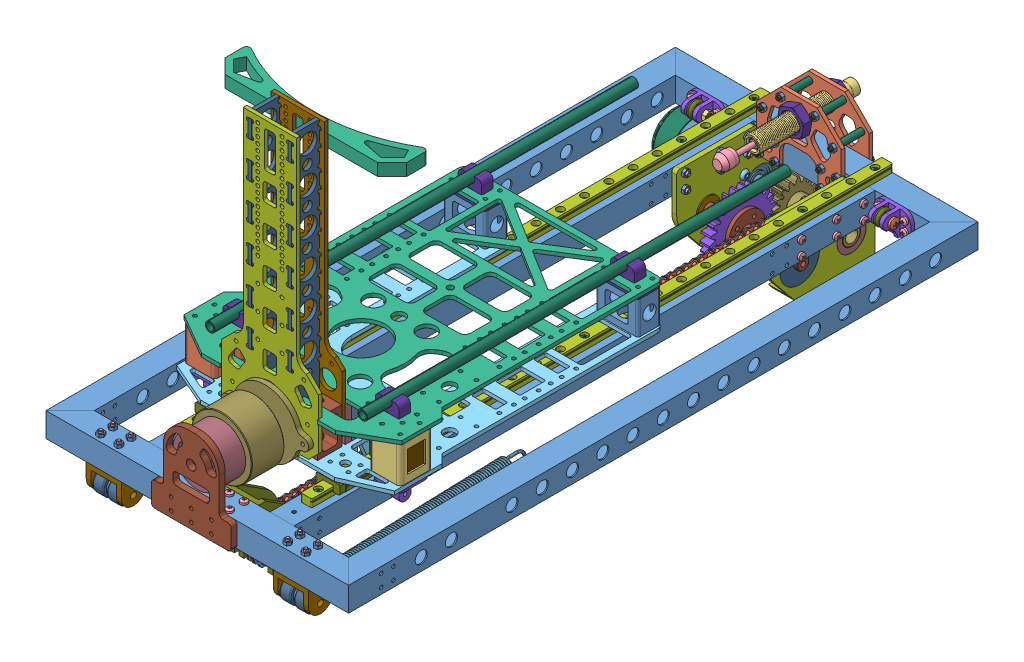
SolidWorks assembly 寒冰射手-wlⅡ-2AT-sc, configuration 默认. Lengths in mm. (continued)
Mates (geometry in assembly coordinates): (continued)
- 同心85: concentric anti-aligned: cylinder of 发射架-wlⅡ-2AT-sc-1 through (-111.2492 36.8186 -178.5) axis (1 0 0) radius 1.5; cylinder of GB／T818-2000十字槽盘头螺钉M3×28-wlⅡ-2AT-sc-7 through (-114.981 36.8186 -178.5) axis (-1 0 0) radius 1.5
- 重合126: coincident anti-aligned: plane of 发射架-wlⅡ-2AT-sc-1 through (-111.2492 32.8186 250) normal (-1 0 0); plane of GB／T818-2000十字槽盘头螺钉M3×28-wlⅡ-2AT-sc-7 through (-111.2492 38.6176 -178.4412) normal (1 0 0)
- 同心86: concentric anti-aligned: cylinder of 发射架-wlⅡ-2AT-sc-1 through (-111.2492 48.8186 -178.5) axis (1 0 0) radius 1.5; cylinder of GB／T818-2000十字槽盘头螺钉M3×28-wlⅡ-2AT-sc-8 through (-114.981 48.8186 -178.5) axis (-1 0 0) radius 1.5
- 同心87: concentric anti-aligned: cylinder of 发射架-wlⅡ-2AT-sc-1 through (-111.2492 48.8186 -207.5) axis (1 0 0) radius 1.5; cylinder of GB／T818-2000十字槽盘头螺钉M3×28-wlⅡ-2AT-sc-10 through (-114.981 48.8186 -207.5) axis (-1 0 0) radius 1.5
- 重合129: coincident anti-aligned: plane of 发射架-wlⅡ-2AT-sc-1 through (-111.2492 32.8186 250) normal (-1 0 0); plane of GB／T818-2000十字槽盘头螺钉M3×28-wlⅡ-2AT-sc-10 through (-111.2492 50.6176 -207.4412) normal (1 0 0)
- 重合130: coincident anti-aligned: plane of 发射架-wlⅡ-2AT-sc-1 through (-111.2492 32.8186 250) normal (-1 0 0); plane of GB／T818-2000十字槽盘头螺钉M3×28-wlⅡ-2AT-sc-8 through (-111.2492 50.6176 -178.4412) normal (1 0 0)
- 同心88: concentric anti-aligned: cylinder of 发射架-wlⅡ-2AT-sc-1 through (-111.2492 36.8186 -207.5) axis (1 0 0) radius 1.5; cylinder of GB／T818-2000十字槽盘头螺钉M3×28-wlⅡ-2AT-sc-9 through (-114.981 36.8186 -207.5) axis (-1 0 0) radius 1.5
- 重合131: coincident anti-aligned: plane of 发射架-wlⅡ-2AT-sc-1 through (-111.2492 32.8186 250) normal (-1 0 0); plane of GB／T818-2000十字槽盘头螺钉M3×28-wlⅡ-2AT-sc-9 through (-111.2492 38.6176 -207.4412) normal (1 0 0)
- 同心89: concentric anti-aligned: cylinder of 发射架-wlⅡ-2AT-sc-1 through (-111.2492 48.8186 -230) axis (1 0 0) radius 1.5; cylinder of GB／T818-2000十字槽盘头螺钉M3×28-wlⅡ-2AT-sc-11 through (-114.981 48.8186 -230) axis (-1 0 0) radius 1.5
- 重合132: coincident anti-aligned: plane of 发射架-wlⅡ-2AT-sc-1 through (-111.2492 32.8186 250) normal (-1 0 0); plane of GB／T818-2000十字槽盘头螺钉M3×28-wlⅡ-2AT-sc-11 through (-111.2492 50.6176 -230.0576) normal (1 0 0)
- 同心90: concentric anti-aligned: cylinder of 发射架-wlⅡ-2AT-sc-1 through (-111.2492 36.8186 -230) axis (1 0 0) radius 1.5; cylinder of GB／T818-2000十字槽盘头螺钉M3×28-wlⅡ-2AT-sc-12 through (-114.981 36.8186 -230) axis (-1 0 0) radius 1.5
- 重合133: coincident anti-aligned: plane of 发射架-wlⅡ-2AT-sc-1 through (-111.2492 32.8186 250) normal (-1 0 0); plane of GB／T818-2000十字槽盘头螺钉M3×28-wlⅡ-2AT-sc-12 through (-111.2492 38.6176 -229.9412) normal (1 0 0)
- 同心91: concentric anti-aligned: cylinder of GB／T818-2000十字槽盘头螺钉M3×28-wlⅡ-2AT-sc-1 through (12.4826 48.8186 -230) axis (1 0 0) radius 1.5; cylinder of GB／T6170-20001型六角螺母A级和B级M3-wlⅡ-2AT-sc-15 through (-15.2492 48.8186 -230) axis (-1 0 0) radius 1.5
- 同心92: concentric anti-aligned: cylinder of GB／T818-2000十字槽盘头螺钉M3×28-wlⅡ-2AT-sc-2 through (12.4826 36.8186 -230) axis (1 0 0) radius 1.5; cylinder of GB／T6170-20001型六角螺母A级和B级M3-wlⅡ-2AT-sc-16 through (-15.2492 36.8186 -230) axis (-1 0 0) radius 1.5
- 同心93: concentric anti-aligned: cylinder of GB／T818-2000十字槽盘头螺钉M3×28-wlⅡ-2AT-sc-3 through (12.4826 36.8186 -207.5) axis (1 0 0) radius 1.5; cylinder of GB／T6170-20001型六角螺母A级和B级M3-wlⅡ-2AT-sc-18 through (-15.2492 36.8186 -207.5) axis (-1 0 0) radius 1.5
- 同心94: concentric anti-aligned: cylinder of GB／T818-2000十字槽盘头螺钉M3×28-wlⅡ-2AT-sc-4 through (12.4826 48.8186 -207.5) axis (1 0 0) radius 1.5; cylinder of GB／T6170-20001型六角螺母A级和B级M3-wlⅡ-2AT-sc-17 through (-15.2492 48.8186 -207.5) axis (-1 0 0) radius 1.5
- 同心95: concentric anti-aligned: cylinder of GB／T818-2000十字槽盘头螺钉M3×28-wlⅡ-2AT-sc-6 through (12.4826 36.8186 -178.5) axis (1 0 0) radius 1.5; cylinder of GB／T6170-20001型六角螺母A级和B级M3-wlⅡ-2AT-sc-20 through (-15.2492 36.8186 -178.5) axis (-1 0 0) radius 1.5
- 同心96: concentric anti-aligned: cylinder of GB／T818-2000十字槽盘头螺钉M3×28-wlⅡ-2AT-sc-5 through (12.4826 48.8186 -178.5) axis (1 0 0) radius 1.5; cylinder of GB／T6170-20001型六角螺母A级和B级M3-wlⅡ-2AT-sc-19 through (-15.2492 48.8186 -178.5) axis (-1 0 0) radius 1.5
- 同心97: concentric aligned: cylinder of GB／T818-2000十字槽盘头螺钉M3×28-wlⅡ-2AT-sc-8 through (-114.981 48.8186 -178.5) axis (-1 0 0) radius 1.5; cylinder of GB／T6170-20001型六角螺母A级和B级M3-wlⅡ-2AT-sc-21 through (-84.8492 48.8186 -178.5) axis (-1 0 0) radius 1.5
- 同心98: concentric aligned: cylinder of GB／T818-2000十字槽盘头螺钉M3×28-wlⅡ-2AT-sc-7 through (-114.981 36.8186 -178.5) axis (-1 0 0) radius 1.5; cylinder of GB／T6170-20001型六角螺母A级和B级M3-wlⅡ-2AT-sc-23 through (-84.8492 36.8186 -178.5) axis (-1 0 0) radius 1.5
- 同心99: concentric aligned: cylinder of GB／T818-2000十字槽盘头螺钉M3×28-wlⅡ-2AT-sc-9 through (-114.981 36.8186 -207.5) axis (-1 0 0) radius 1.5; cylinder of GB／T6170-20001型六角螺母A级和B级M3-wlⅡ-2AT-sc-28 through (-84.8492 36.8186 -207.5) axis (-1 0 0) radius 1.5
- 同心100: concentric aligned: cylinder of GB／T818-2000十字槽盘头螺钉M3×28-wlⅡ-2AT-sc-10 through (-114.981 48.8186 -207.5) axis (-1 0 0) radius 1.5; cylinder of GB／T6170-20001型六角螺母A级和B级M3-wlⅡ-2AT-sc-26 through (-84.8492 48.8186 -207.5) axis (-1 0 0) radius 1.5
- 同心101: concentric aligned: cylinder of GB／T818-2000十字槽盘头螺钉M3×28-wlⅡ-2AT-sc-11 through (-114.981 48.8186 -230) axis (-1 0 0) radius 1.5; cylinder of GB／T6170-20001型六角螺母A级和B级M3-wlⅡ-2AT-sc-27 through (-84.8492 48.8186 -230) axis (-1 0 0) radius 1.5
- 同心102: concentric aligned: cylinder of GB／T818-2000十字槽盘头螺钉M3×28-wlⅡ-2AT-sc-12 through (-114.981 36.8186 -230) axis (-1 0 0) radius 1.5; cylinder of GB／T6170-20001型六角螺母A级和B级M3-wlⅡ-2AT-sc-24 through (-84.8492 36.8186 -230) axis (-1 0 0) radius 1.5
- 同心107: concentric anti-aligned: cylinder of 拉线座子-wlⅡ-2AT-sc-2 through (-117.7492 46.8186 -237) axis (0 0 -1) radius 1.5; cylinder of GB／T818-2000十字槽盘头螺钉M3×28-wlⅡ-2AT-sc-13 through (-117.7492 46.8186 -233.2682) axis (0 0 1) radius 1.5
- 重合153: coincident anti-aligned: plane of 拉线座子-wlⅡ-2AT-sc-2 through (-128.4992 25.8186 -237) normal (0 0 1); plane of GB／T818-2000十字槽盘头螺钉M3×28-wlⅡ-2AT-sc-13 through (-118.3588 48.5122 -237) normal (0 0 -1)
- 同心108: concentric anti-aligned: cylinder of 拉线座子-wlⅡ-2AT-sc-2 through (-139.2492 46.8186 -237) axis (0 0 -1) radius 1.5; cylinder of GB／T818-2000十字槽盘头螺钉M3×28-wlⅡ-2AT-sc-16 through (-139.2492 46.8186 -233.2682) axis (0 0 1) radius 1.5
- 同心109: concentric anti-aligned: cylinder of 拉线座子-wlⅡ-2AT-sc-2 through (-139.2492 38.8186 -237) axis (0 0 -1) radius 1.5; cylinder of GB／T818-2000十字槽盘头螺钉M3×28-wlⅡ-2AT-sc-14 through (-139.2492 38.8186 -233.2682) axis (0 0 1) radius 1.5
- 同心110: concentric anti-aligned: cylinder of 拉线座子-wlⅡ-2AT-sc-2 through (-117.7492 38.8186 -237) axis (0 0 -1) radius 1.5; cylinder of GB／T818-2000十字槽盘头螺钉M3×28-wlⅡ-2AT-sc-15 through (-117.7492 38.8186 -233.2682) axis (0 0 1) radius 1.5
- 重合154: coincident anti-aligned: plane of 拉线座子-wlⅡ-2AT-sc-2 through (-128.4992 25.8186 -237) normal (0 0 1); plane of GB／T818-2000十字槽盘头螺钉M3×28-wlⅡ-2AT-sc-15 through (-118.3588 40.5122 -237) normal (0 0 -1)
- 重合155: coincident anti-aligned: plane of 拉线座子-wlⅡ-2AT-sc-2 through (-128.4992 25.8186 -237) normal (0 0 1); plane of GB／T818-2000十字槽盘头螺钉M3×28-wlⅡ-2AT-sc-16 through (-139.8588 48.5122 -237) normal (0 0 -1)
- 重合156: coincident anti-aligned: plane of 拉线座子-wlⅡ-2AT-sc-2 through (-128.4992 25.8186 -237) normal (0 0 1); plane of GB／T818-2000十字槽盘头螺钉M3×28-wlⅡ-2AT-sc-14 through (-139.8588 40.5122 -237) normal (0 0 -1)
- 同心111: concentric anti-aligned: cylinder of 拉线座子-wlⅡ-2AT-sc-1 through (15.2508 46.8186 -237) axis (0 0 -1) radius 1.5; cylinder of GB／T818-2000十字槽盘头螺钉M3×28-wlⅡ-2AT-sc-17 through (15.2508 46.8186 -233.2682) axis (0 0 1) radius 1.5
- 同心112: concentric anti-aligned: cylinder of 拉线座子-wlⅡ-2AT-sc-1 through (15.2508 38.8186 -237) axis (0 0 -1) radius 1.5; cylinder of GB／T818-2000十字槽盘头螺钉M3×28-wlⅡ-2AT-sc-19 through (15.2508 38.8186 -233.2682) axis (0 0 1) radius 1.5
- 同心113: concentric anti-aligned: cylinder of 拉线座子-wlⅡ-2AT-sc-1 through (36.7508 38.8186 -237) axis (0 0 -1) radius 1.5; cylinder of GB／T818-2000十字槽盘头螺钉M3×28-wlⅡ-2AT-sc-20 through (36.7508 38.8186 -233.2682) axis (0 0 1) radius 1.5
- 同心114: concentric anti-aligned: cylinder of 拉线座子-wlⅡ-2AT-sc-1 through (36.7508 46.8186 -237) axis (0 0 -1) radius 1.5; cylinder of GB／T818-2000十字槽盘头螺钉M3×28-wlⅡ-2AT-sc-18 through (36.7508 46.8186 -233.2682) axis (0 0 1) radius 1.5
- 重合157: coincident anti-aligned: plane of 拉线座子-wlⅡ-2AT-sc-1 through (26.0008 25.8186 -237) normal (0 0 1); plane of GB／T818-2000十字槽盘头螺钉M3×28-wlⅡ-2AT-sc-19 through (14.6412 40.5122 -237) normal (0 0 -1)
- 重合158: coincident anti-aligned: plane of 拉线座子-wlⅡ-2AT-sc-1 through (26.0008 25.8186 -237) normal (0 0 1); plane of GB／T818-2000十字槽盘头螺钉M3×28-wlⅡ-2AT-sc-18 through (36.1412 48.5122 -237) normal (0 0 -1)
- 重合159: coincident anti-aligned: plane of 拉线座子-wlⅡ-2AT-sc-1 through (26.0008 25.8186 -237) normal (0 0 1); plane of GB／T818-2000十字槽盘头螺钉M3×28-wlⅡ-2AT-sc-20 through (36.1412 40.5122 -237) normal (0 0 -1)
- 同心115: concentric anti-aligned: cylinder of GB／T818-2000十字槽盘头螺钉M3×28-wlⅡ-2AT-sc-20 through (36.7508 38.8186 -233.2682) axis (0 0 1) radius 1.5; cylinder of GB／T6170-20001型六角螺母A级和B级M3-wlⅡ-2AT-sc-29 through (36.7508 38.8186 -260) axis (0 0 -1) radius 1.5
- 重合160: coincident anti-aligned: plane of 发射架-wlⅡ-2AT-sc-1 through (63.7508 32.8186 -260) normal (0 0 -1); plane of GB／T6170-20001型六角螺母A级和B级M3-wlⅡ-2AT-sc-29 through (33.7458 38.8186 -260) normal (0 0 1)
- 同心116: concentric anti-aligned: cylinder of GB／T818-2000十字槽盘头螺钉M3×28-wlⅡ-2AT-sc-18 through (36.7508 46.8186 -233.2682) axis (0 0 1) radius 1.5; cylinder of GB／T6170-20001型六角螺母A级和B级M3-wlⅡ-2AT-sc-30 through (36.7508 46.8186 -260) axis (0 0 -1) radius 1.5
- 重合161: coincident anti-aligned: plane of 发射架-wlⅡ-2AT-sc-1 through (63.7508 32.8186 -260) normal (0 0 -1); plane of GB／T6170-20001型六角螺母A级和B级M3-wlⅡ-2AT-sc-30 through (33.7458 46.8186 -260) normal (0 0 1)
- 同心117: concentric anti-aligned: cylinder of GB／T818-2000十字槽盘头螺钉M3×28-wlⅡ-2AT-sc-19 through (15.2508 38.8186 -233.2682) axis (0 0 1) radius 1.5; cylinder of GB／T6170-20001型六角螺母A级和B级M3-wlⅡ-2AT-sc-31 through (15.2508 38.8186 -260) axis (0 0 -1) radius 1.5
- 同心118: concentric anti-aligned: cylinder of GB／T818-2000十字槽盘头螺钉M3×28-wlⅡ-2AT-sc-17 through (15.2508 46.8186 -233.2682) axis (0 0 1) radius 1.5; cylinder of GB／T6170-20001型六角螺母A级和B级M3-wlⅡ-2AT-sc-32 through (15.2508 46.8186 -260) axis (0 0 -1) radius 1.5
- 重合162: coincident anti-aligned: plane of 发射架-wlⅡ-2AT-sc-1 through (63.7508 32.8186 -260) normal (0 0 -1); plane of GB／T6170-20001型六角螺母A级和B级M3-wlⅡ-2AT-sc-32 through (12.2458 46.8186 -260) normal (0 0 1)
- 重合163: coincident anti-aligned: plane of 发射架-wlⅡ-2AT-sc-1 through (63.7508 32.8186 -260) normal (0 0 -1); plane of GB／T6170-20001型六角螺母A级和B级M3-wlⅡ-2AT-sc-31 through (12.2458 38.8186 -260) normal (0 0 1)
- 同心119: concentric anti-aligned: cylinder of GB／T818-2000十字槽盘头螺钉M3×28-wlⅡ-2AT-sc-15 through (-117.7492 38.8186 -233.2682) axis (0 0 1) radius 1.5; cylinder of GB／T6170-20001型六角螺母A级和B级M3-wlⅡ-2AT-sc-33 through (-117.7492 38.8186 -260) axis (0 0 -1) radius 1.5
- 同心120: concentric anti-aligned: cylinder of GB／T818-2000十字槽盘头螺钉M3×28-wlⅡ-2AT-sc-13 through (-117.7492 46.8186 -233.2682) axis (0 0 1) radius 1.5; cylinder of GB／T6170-20001型六角螺母A级和B级M3-wlⅡ-2AT-sc-35 through (-117.7492 46.8186 -260) axis (0 0 -1) radius 1.5
- 同心121: concentric anti-aligned: cylinder of GB／T818-2000十字槽盘头螺钉M3×28-wlⅡ-2AT-sc-14 through (-139.2492 38.8186 -233.2682) axis (0 0 1) radius 1.5; cylinder of GB／T6170-20001型六角螺母A级和B级M3-wlⅡ-2AT-sc-34 through (-139.2492 38.8186 -260) axis (0 0 -1) radius 1.5
- 同心122: concentric anti-aligned: cylinder of GB／T818-2000十字槽盘头螺钉M3×28-wlⅡ-2AT-sc-16 through (-139.2492 46.8186 -233.2682) axis (0 0 1) radius 1.5; cylinder of GB／T6170-20001型六角螺母A级和B级M3-wlⅡ-2AT-sc-36 through (-139.2492 46.8186 -260) axis (0 0 -1) radius 1.5
- 重合164: coincident anti-aligned: plane of 发射架-wlⅡ-2AT-sc-1 through (63.7508 32.8186 -260) normal (0 0 -1); plane of GB／T6170-20001型六角螺母A级和B级M3-wlⅡ-2AT-sc-35 through (-120.7542 46.8186 -260) normal (0 0 1)
- 重合165: coincident anti-aligned: plane of 发射架-wlⅡ-2AT-sc-1 through (63.7508 32.8186 -260) normal (0 0 -1); plane of GB／T6170-20001型六角螺母A级和B级M3-wlⅡ-2AT-sc-33 through (-120.7542 38.8186 -260) normal (0 0 1)
- 重合166: coincident anti-aligned: plane of 发射架-wlⅡ-2AT-sc-1 through (63.7508 32.8186 -260) normal (0 0 -1); plane of GB／T6170-20001型六角螺母A级和B级M3-wlⅡ-2AT-sc-36 through (-142.2542 46.8186 -260) normal (0 0 1)
- 重合167: coincident anti-aligned: plane of 发射架-wlⅡ-2AT-sc-1 through (63.7508 32.8186 -260) normal (0 0 -1); plane of GB／T6170-20001型六角螺母A级和B级M3-wlⅡ-2AT-sc-34 through (-142.2542 38.8186 -260) normal (0 0 1)
- 同心123: concentric aligned: cylinder of 发射导轨-wlⅡ-2AT-sc-1 through (-1.2492 52.8186 -190) axis (0 1 0) radius 1.75; cylinder of GB／T818-2000十字槽盘头螺钉M3×25-wlⅡ-2AT-sc-1 through (-1.2492 59.5503 -190) axis (0 1 0) radius 1.5
- 重合168: coincident anti-aligned: plane of 发射导轨-wlⅡ-2AT-sc-1 through (-1.2492 55.8186 -190) normal (0 1 0); plane of GB／T818-2000十字槽盘头螺钉M3×25-wlⅡ-2AT-sc-1 through (0.371 55.8186 -189.2159) normal (0 -1 0)
- 同心124: concentric aligned: cylinder of 发射导轨-wlⅡ-2AT-sc-2 through (-101.2492 52.8186 -190) axis (0 1 0) radius 1.75; cylinder of GB／T818-2000十字槽盘头螺钉M3×25-wlⅡ-2AT-sc-2 through (-101.2492 59.5503 -190) axis (0 1 0) radius 1.5
- 重合169: coincident anti-aligned: plane of 发射导轨-wlⅡ-2AT-sc-2 through (-101.2492 55.8186 -190) normal (0 1 0); plane of GB／T818-2000十字槽盘头螺钉M3×25-wlⅡ-2AT-sc-2 through (-101.0011 55.8186 -188.2172) normal (0 -1 0)
- 同心125: concentric aligned: cylinder of 发射导轨-wlⅡ-2AT-sc-2 through (-101.2492 52.8186 -250) axis (0 1 0) radius 1.75; cylinder of GB／T818-2000十字槽盘头螺钉M3×25-wlⅡ-2AT-sc-3 through (-101.2492 59.5503 -250) axis (0 1 0) radius 1.5
- 重合170: coincident anti-aligned: plane of 发射导轨-wlⅡ-2AT-sc-2 through (-101.2492 55.8186 -250) normal (0 1 0); plane of GB／T818-2000十字槽盘头螺钉M3×25-wlⅡ-2AT-sc-3 through (-100.9482 55.8186 -251.7747) normal (0 -1 0)
- 同心126: concentric aligned: cylinder of 发射导轨-wlⅡ-2AT-sc-2 through (-101.2492 52.8186 210) axis (0 1 0) radius 1.75; cylinder of GB／T818-2000十字槽盘头螺钉M3×25-wlⅡ-2AT-sc-8 through (-101.2492 59.5503 210) axis (0 1 0) radius 1.5
- 重合171: coincident anti-aligned: plane of 发射导轨-wlⅡ-2AT-sc-2 through (-101.2492 55.8186 210) normal (0 1 0); plane of GB／T818-2000十字槽盘头螺钉M3×25-wlⅡ-2AT-sc-8 through (-100.9482 55.8186 208.2253) normal (0 -1 0)
- 同心128: concentric aligned: cylinder of 发射导轨-wlⅡ-2AT-sc-1 through (-1.2492 52.8186 210) axis (0 1 0) radius 1.75; cylinder of GB／T818-2000十字槽盘头螺钉M3×25-wlⅡ-2AT-sc-7 through (-1.2492 59.5503 210) axis (0 1 0) radius 1.5
- 重合172: coincident anti-aligned: plane of 发射导轨-wlⅡ-2AT-sc-1 through (-1.2492 55.8186 210) normal (0 1 0); plane of GB／T818-2000十字槽盘头螺钉M3×25-wlⅡ-2AT-sc-7 through (-0.9482 55.8186 208.2253) normal (0 -1 0)
- 同心129: concentric aligned: cylinder of 发射导轨-wlⅡ-2AT-sc-2 through (-101.2492 52.8186 -10) axis (0 1 0) radius 1.75; cylinder of GB／T818-2000十字槽盘头螺钉M3×25-wlⅡ-2AT-sc-6 through (-101.2492 59.5503 -10) axis (0 1 0) radius 1.5
- 重合173: coincident anti-aligned: plane of 发射导轨-wlⅡ-2AT-sc-2 through (-101.2492 55.8186 -10) normal (0 1 0); plane of GB／T818-2000十字槽盘头螺钉M3×25-wlⅡ-2AT-sc-6 through (-100.9482 55.8186 -11.7747) normal (0 -1 0)
- 同心130: concentric aligned: cylinder of 发射导轨-wlⅡ-2AT-sc-1 through (-1.2492 52.8186 -10) axis (0 1 0) radius 1.75; cylinder of GB／T818-2000十字槽盘头螺钉M3×25-wlⅡ-2AT-sc-5 through (-1.2492 59.5503 -10) axis (0 1 0) radius 1.5
- 重合174: coincident anti-aligned: plane of 发射导轨-wlⅡ-2AT-sc-1 through (-1.2492 55.8186 -10) normal (0 1 0); plane of GB／T818-2000十字槽盘头螺钉M3×25-wlⅡ-2AT-sc-5 through (-2.3845 55.8186 -11.3968) normal (0 -1 0)
- 同心131: concentric anti-aligned: cylinder of GB／T818-2000十字槽盘头螺钉M3×25-wlⅡ-2AT-sc-2 through (-101.2492 59.5503 -190) axis (0 1 0) radius 1.5; cylinder of GB／T6170-20001型六角螺母A级和B级M3-wlⅡ-2AT-sc-37 through (-101.2492 32.8186 -190) axis (0 -1 0) radius 1.5
- 重合177: coincident anti-aligned: plane of 发射架-wlⅡ-2AT-sc-1 through (-111.2492 32.8186 250) normal (0 -1 0); plane of GB／T6170-20001型六角螺母A级和B级M3-wlⅡ-2AT-sc-37 through (-102.7414 32.8186 -192.6083) normal (0 1 0)
- 重合178: coincident anti-aligned: plane of 发射导轨-wlⅡ-2AT-sc-1 through (-1.2492 55.8186 -250) normal (0 1 0); plane of GB／T818-2000十字槽盘头螺钉M3×25-wlⅡ-2AT-sc-4 through (0.4005 55.8186 -249.28) normal (0 -1 0)
- 同心133: concentric anti-aligned: cylinder of GB／T818-2000十字槽盘头螺钉M3×25-wlⅡ-2AT-sc-4 through (-1.2492 59.5503 -250) axis (0 1 0) radius 1.5; cylinder of GB／T6170-20001型六角螺母A级和B级M3-wlⅡ-2AT-sc-39 through (-1.2492 32.8186 -250) axis (0 -1 0) radius 1.5
- 重合179: coincident anti-aligned: plane of 发射架-wlⅡ-2AT-sc-1 through (63.7508 32.8186 -240) normal (0 -1 0); plane of GB／T6170-20001型六角螺母A级和B级M3-wlⅡ-2AT-sc-39 through (-2.7414 32.8186 -252.6083) normal (0 1 0)
- 同心134: concentric anti-aligned: cylinder of GB／T818-2000十字槽盘头螺钉M3×25-wlⅡ-2AT-sc-3 through (-101.2492 59.5503 -250) axis (0 1 0) radius 1.5; cylinder of GB／T6170-20001型六角螺母A级和B级M3-wlⅡ-2AT-sc-38 through (-101.2492 32.8186 -250) axis (0 -1 0) radius 1.5
- 重合180: coincident anti-aligned: plane of 发射架-wlⅡ-2AT-sc-1 through (63.7508 32.8186 -240) normal (0 -1 0); plane of GB／T6170-20001型六角螺母A级和B级M3-wlⅡ-2AT-sc-38 through (-102.7414 32.8186 -252.6083) normal (0 1 0)
- 同心135: concentric anti-aligned: cylinder of GB／T818-2000十字槽盘头螺钉M3×25-wlⅡ-2AT-sc-8 through (-101.2492 59.5503 210) axis (0 1 0) radius 1.5; cylinder of GB／T6170-20001型六角螺母A级和B级M3-wlⅡ-2AT-sc-43 through (-101.2492 32.8186 210) axis (0 -1 0) radius 1.5
- 重合181: coincident anti-aligned: plane of 发射架-wlⅡ-2AT-sc-1 through (-111.2492 32.8186 250) normal (0 -1 0); plane of GB／T6170-20001型六角螺母A级和B级M3-wlⅡ-2AT-sc-43 through (-102.7414 32.8186 207.3917) normal (0 1 0)
- 同心136: concentric anti-aligned: cylinder of GB／T818-2000十字槽盘头螺钉M3×25-wlⅡ-2AT-sc-7 through (-1.2492 59.5503 210) axis (0 1 0) radius 1.5; cylinder of GB／T6170-20001型六角螺母A级和B级M3-wlⅡ-2AT-sc-44 through (-1.2492 32.8186 210) axis (0 -1 0) radius 1.5
- 重合182: coincident anti-aligned: plane of 发射架-wlⅡ-2AT-sc-1 through (-11.2492 32.8186 250) normal (0 -1 0); plane of GB／T6170-20001型六角螺母A级和B级M3-wlⅡ-2AT-sc-44 through (-2.7414 32.8186 207.3917) normal (0 1 0)
- 同心137: concentric anti-aligned: cylinder of GB／T818-2000十字槽盘头螺钉M3×25-wlⅡ-2AT-sc-6 through (-101.2492 59.5503 -10) axis (0 1 0) radius 1.5; cylinder of GB／T6170-20001型六角螺母A级和B级M3-wlⅡ-2AT-sc-42 through (-101.2492 32.8186 -10) axis (0 -1 0) radius 1.5
- 重合183: coincident anti-aligned: plane of 发射架-wlⅡ-2AT-sc-1 through (-111.2492 32.8186 250) normal (0 -1 0); plane of GB／T6170-20001型六角螺母A级和B级M3-wlⅡ-2AT-sc-42 through (-102.7414 32.8186 -12.6083) normal (0 1 0)
- 重合184: coincident anti-aligned: plane of 发射架-wlⅡ-2AT-sc-1 through (-11.2492 32.8186 250) normal (0 -1 0); plane of GB／T6170-20001型六角螺母A级和B级M3-wlⅡ-2AT-sc-41 through (-2.7414 32.8186 -12.6083) normal (0 1 0)
- 同心138: concentric anti-aligned: cylinder of GB／T818-2000十字槽盘头螺钉M3×25-wlⅡ-2AT-sc-5 through (-1.2492 59.5503 -10) axis (0 1 0) radius 1.5; cylinder of GB／T6170-20001型六角螺母A级和B级M3-wlⅡ-2AT-sc-41 through (-1.2492 32.8186 -10) axis (0 -1 0) radius 1.5
- 同心139: concentric anti-aligned: cylinder of GB／T818-2000十字槽盘头螺钉M3×25-wlⅡ-2AT-sc-1 through (-1.2492 59.5503 -190) axis (0 1 0) radius 1.5; cylinder of GB／T6170-20001型六角螺母A级和B级M3-wlⅡ-2AT-sc-40 through (-1.2492 32.8186 -190) axis (0 -1 0) radius 1.5
- 重合185: coincident anti-aligned: plane of 发射架-wlⅡ-2AT-sc-1 through (-11.2492 32.8186 250) normal (0 -1 0); plane of GB／T6170-20001型六角螺母A级和B级M3-wlⅡ-2AT-sc-40 through (-2.7414 32.8186 -192.6083) normal (0 1 0)
- 重合186: coincident anti-aligned: plane of 拉簧座子-wlⅡ-2AT-sc-2 through (-128.4992 28.8186 250) normal (0 -1 0); plane of GB／T818-2000十字槽盘头螺钉M3×28-wlⅡ-2AT-sc-21 through (-137.7982 28.8186 245.0588) normal (0 1 0)
- 同心141: concentric anti-aligned: cylinder of 拉簧座子-wlⅡ-2AT-sc-2 through (-135.9992 28.8186 255) axis (0 1 0) radius 1.5; cylinder of GB／T818-2000十字槽盘头螺钉M3×28-wlⅡ-2AT-sc-22 through (-135.9992 25.0868 255) axis (0 -1 0) radius 1.5
- 重合187: coincident anti-aligned: plane of 拉簧座子-wlⅡ-2AT-sc-2 through (-128.4992 28.8186 250) normal (0 -1 0); plane of GB／T818-2000十字槽盘头螺钉M3×28-wlⅡ-2AT-sc-22 through (-137.7982 28.8186 255.0588) normal (0 1 0)
- 同心142: concentric anti-aligned: cylinder of 拉簧座子-wlⅡ-2AT-sc-2 through (-120.9992 28.8186 255) axis (0 1 0) radius 1.5; cylinder of GB／T818-2000十字槽盘头螺钉M3×28-wlⅡ-2AT-sc-23 through (-120.9992 25.0868 255) axis (0 -1 0) radius 1.5
- 重合188: coincident anti-aligned: plane of 拉簧座子-wlⅡ-2AT-sc-2 through (-128.4992 28.8186 250) normal (0 -1 0); plane of GB／T818-2000十字槽盘头螺钉M3×28-wlⅡ-2AT-sc-23 through (-122.7982 28.8186 255.0588) normal (0 1 0)
- 同心143: concentric anti-aligned: cylinder of 拉簧座子-wlⅡ-2AT-sc-2 through (-120.9992 28.8186 245) axis (0 1 0) radius 1.5; cylinder of GB／T818-2000十字槽盘头螺钉M3×28-wlⅡ-2AT-sc-24 through (-120.9992 25.0868 245) axis (0 -1 0) radius 1.5
- 重合189: coincident anti-aligned: plane of 拉簧座子-wlⅡ-2AT-sc-2 through (-128.4992 28.8186 250) normal (0 -1 0); plane of GB／T818-2000十字槽盘头螺钉M3×28-wlⅡ-2AT-sc-24 through (-122.2207 28.8186 243.6779) normal (0 1 0)
- 同心144: concentric anti-aligned: cylinder of 拉簧座子-wlⅡ-2AT-sc-1 through (18.5008 28.8186 255) axis (0 1 0) radius 1.5; cylinder of GB／T818-2000十字槽盘头螺钉M3×28-wlⅡ-2AT-sc-25 through (18.5008 25.0868 255) axis (0 -1 0) radius 1.5
- 重合190: coincident anti-aligned: plane of 拉簧座子-wlⅡ-2AT-sc-1 through (26.0008 28.8186 250) normal (0 -1 0); plane of GB／T818-2000十字槽盘头螺钉M3×28-wlⅡ-2AT-sc-25 through (16.7018 28.8186 255.0588) normal (0 1 0)
- 同心145: concentric anti-aligned: cylinder of 拉簧座子-wlⅡ-2AT-sc-1 through (33.5008 28.8186 255) axis (0 1 0) radius 1.5; cylinder of GB／T818-2000十字槽盘头螺钉M3×28-wlⅡ-2AT-sc-27 through (33.5008 25.0868 255) axis (0 -1 0) radius 1.5
- 重合191: coincident anti-aligned: plane of 拉簧座子-wlⅡ-2AT-sc-1 through (26.0008 28.8186 250) normal (0 -1 0); plane of GB／T818-2000十字槽盘头螺钉M3×28-wlⅡ-2AT-sc-27 through (31.7018 28.8186 255.0588) normal (0 1 0)
- 重合193: coincident anti-aligned: plane of 拉簧座子-wlⅡ-2AT-sc-1 through (26.0008 28.8186 250) normal (0 -1 0); plane of GB／T818-2000十字槽盘头螺钉M3×28-wlⅡ-2AT-sc-28 through (16.7018 28.8186 245.0588) normal (0 1 0)
- 重合194: coincident anti-aligned: plane of 拉簧座子-wlⅡ-2AT-sc-1 through (26.0008 28.8186 250) normal (0 -1 0); plane of GB／T818-2000十字槽盘头螺钉M3×28-wlⅡ-2AT-sc-26 through (31.7018 28.8186 245.0588) normal (0 1 0)
- 同心147: concentric anti-aligned: cylinder of 拉簧座子-wlⅡ-2AT-sc-1 through (33.5008 28.8186 245) axis (0 1 0) radius 1.5; cylinder of GB／T818-2000十字槽盘头螺钉M3×28-wlⅡ-2AT-sc-26 through (33.5008 25.0868 245) axis (0 -1 0) radius 1.5
- 同心148: concentric anti-aligned: cylinder of 拉簧座子-wlⅡ-2AT-sc-1 through (18.5008 28.8186 245) axis (0 1 0) radius 1.5; cylinder of GB／T818-2000十字槽盘头螺钉M3×28-wlⅡ-2AT-sc-28 through (18.5008 25.0868 245) axis (0 -1 0) radius 1.5
- 重合196: coincident anti-aligned: plane of 发射架-wlⅡ-2AT-sc-1 through (-166.2492 52.8186 240) normal (0 1 0); plane of GB／T818-2000十字槽盘头螺钉M3×28-wlⅡ-2AT-sc-29 through (-27.1752 52.8186 245.0332) normal (0 -1 0)
- 重合197: coincident anti-aligned: plane of 发射架-wlⅡ-2AT-sc-1 through (-166.2492 52.8186 240) normal (0 1 0); plane of GB／T818-2000十字槽盘头螺钉M3×28-wlⅡ-2AT-sc-30 through (-40.5723 52.8186 242.2016) normal (0 -1 0)
- 重合198: coincident anti-aligned: plane of 发射架-wlⅡ-2AT-sc-1 through (-166.2492 52.8186 240) normal (0 1 0); plane of GB／T818-2000十字槽盘头螺钉M3×28-wlⅡ-2AT-sc-32 through (-27.1752 52.8186 257.0332) normal (0 -1 0)
- 重合199: coincident anti-aligned: plane of 发射架-wlⅡ-2AT-sc-1 through (-166.2492 52.8186 240) normal (0 1 0); plane of GB／T818-2000十字槽盘头螺钉M3×28-wlⅡ-2AT-sc-31 through (-39.1752 52.8186 257.0332) normal (0 -1 0)
- 同心153: concentric anti-aligned: cylinder of GB／T818-2000十字槽盘头螺钉M3×28-wlⅡ-2AT-sc-32 through (-28.6492 56.5503 256) axis (0 1 0) radius 1.5; cylinder of GB／T6170-20001型六角螺母A级和B级M3-wlⅡ-2AT-sc-46 through (-28.6492 28.8186 256) axis (0 -1 0) radius 1.5
- 同心154: concentric anti-aligned: cylinder of GB／T818-2000十字槽盘头螺钉M3×28-wlⅡ-2AT-sc-31 through (-40.6492 56.5503 256) axis (0 1 0) radius 1.5; cylinder of GB／T6170-20001型六角螺母A级和B级M3-wlⅡ-2AT-sc-49 through (-40.6492 28.8186 256) axis (0 -1 0) radius 1.5
- 同心155: concentric anti-aligned: cylinder of GB／T818-2000十字槽盘头螺钉M3×28-wlⅡ-2AT-sc-30 through (-40.6492 56.5503 244) axis (0 1 0) radius 1.5; cylinder of GB／T6170-20001型六角螺母A级和B级M3-wlⅡ-2AT-sc-48 through (-40.6492 28.8186 244) axis (0 -1 0) radius 1.5
- 同心156: concentric anti-aligned: cylinder of GB／T818-2000十字槽盘头螺钉M3×28-wlⅡ-2AT-sc-29 through (-28.6492 56.5503 244) axis (0 1 0) radius 1.5; cylinder of GB／T6170-20001型六角螺母A级和B级M3-wlⅡ-2AT-sc-47 through (-28.6492 28.8186 244) axis (0 -1 0) radius 1.5
- 同心157: concentric aligned: cylinder of GB／T818-2000十字槽盘头螺钉M3×28-wlⅡ-2AT-sc-27 through (33.5008 25.0868 255) axis (0 -1 0) radius 1.5; cylinder of GB／T6170-20001型六角螺母A级和B级M3-wlⅡ-2AT-sc-53 through (33.5008 55.2186 255) axis (0 -1 0) radius 1.5
- 同心158: concentric aligned: cylinder of GB／T818-2000十字槽盘头螺钉M3×28-wlⅡ-2AT-sc-25 through (18.5008 25.0868 255) axis (0 -1 0) radius 1.5; cylinder of GB／T6170-20001型六角螺母A级和B级M3-wlⅡ-2AT-sc-52 through (18.5008 55.2186 255) axis (0 -1 0) radius 1.5
- 同心159: concentric aligned: cylinder of GB／T818-2000十字槽盘头螺钉M3×28-wlⅡ-2AT-sc-26 through (33.5008 25.0868 245) axis (0 -1 0) radius 1.5; cylinder of GB／T6170-20001型六角螺母A级和B级M3-wlⅡ-2AT-sc-51 through (33.5008 55.2186 245) axis (0 -1 0) radius 1.5
- 同心160: concentric aligned: cylinder of GB／T818-2000十字槽盘头螺钉M3×28-wlⅡ-2AT-sc-28 through (18.5008 25.0868 245) axis (0 -1 0) radius 1.5; cylinder of GB／T6170-20001型六角螺母A级和B级M3-wlⅡ-2AT-sc-50 through (18.5008 55.2186 245) axis (0 -1 0) radius 1.5
- 重合205: coincident anti-aligned: plane of 发射架-wlⅡ-2AT-sc-1 through (-166.2492 52.8186 240) normal (0 1 0); plane of GB／T6170-20001型六角螺母A级和B级M3-wlⅡ-2AT-sc-52 through (16.979 52.8186 252.4088) normal (0 -1 0)
- 重合206: coincident anti-aligned: plane of 发射架-wlⅡ-2AT-sc-1 through (-166.2492 52.8186 240) normal (0 1 0); plane of GB／T6170-20001型六角螺母A级和B级M3-wlⅡ-2AT-sc-53 through (32.0086 52.8186 252.3917) normal (0 -1 0)
- 重合207: coincident anti-aligned: plane of 发射架-wlⅡ-2AT-sc-1 through (-166.2492 52.8186 240) normal (0 1 0); plane of GB／T6170-20001型六角螺母A级和B级M3-wlⅡ-2AT-sc-51 through (32.62 52.8186 247.873) normal (0 -1 0)
- 重合208: coincident anti-aligned: plane of 发射架-wlⅡ-2AT-sc-1 through (-166.2492 52.8186 240) normal (0 1 0); plane of GB／T6170-20001型六角螺母A级和B级M3-wlⅡ-2AT-sc-50 through (18.3227 52.8186 247.9997) normal (0 -1 0)
- 同心161: concentric aligned: cylinder of GB／T818-2000十字槽盘头螺钉M3×28-wlⅡ-2AT-sc-23 through (-120.9992 25.0868 255) axis (0 -1 0) radius 1.5; cylinder of GB／T6170-20001型六角螺母A级和B级M3-wlⅡ-2AT-sc-56 through (-120.9992 55.2186 255) axis (0 -1 0) radius 1.5
- 同心162: concentric aligned: cylinder of GB／T818-2000十字槽盘头螺钉M3×28-wlⅡ-2AT-sc-22 through (-135.9992 25.0868 255) axis (0 -1 0) radius 1.5; cylinder of GB／T6170-20001型六角螺母A级和B级M3-wlⅡ-2AT-sc-54 through (-135.9992 55.2186 255) axis (0 -1 0) radius 1.5
- 重合210: coincident anti-aligned: plane of 发射架-wlⅡ-2AT-sc-1 through (-166.2492 52.8186 240) normal (0 1 0); plane of GB／T6170-20001型六角螺母A级和B级M3-wlⅡ-2AT-sc-56 through (-122.9251 52.8186 257.3067) normal (0 -1 0)
- 重合211: coincident anti-aligned: plane of 发射架-wlⅡ-2AT-sc-1 through (-166.2492 52.8186 240) normal (0 1 0); plane of GB／T6170-20001型六角螺母A级和B级M3-wlⅡ-2AT-sc-54 through (-134.8513 52.8186 257.7771) normal (0 -1 0)
- 同心164: concentric aligned: cylinder of GB／T818-2000十字槽盘头螺钉M3×28-wlⅡ-2AT-sc-21 through (-135.9992 25.0868 245) axis (0 -1 0) radius 1.5; cylinder of GB／T6170-20001型六角螺母A级和B级M3-wlⅡ-2AT-sc-55 through (-135.9992 55.2186 245) axis (0 -1 0) radius 1.5
- 同心165: concentric aligned: cylinder of GB／T818-2000十字槽盘头螺钉M3×28-wlⅡ-2AT-sc-24 through (-120.9992 25.0868 245) axis (0 -1 0) radius 1.5; cylinder of GB／T6170-20001型六角螺母A级和B级M3-wlⅡ-2AT-sc-57 through (-120.9992 55.2186 245) axis (0 -1 0) radius 1.5
- 重合212: coincident anti-aligned: plane of 发射架-wlⅡ-2AT-sc-1 through (-166.2492 52.8186 240) normal (0 1 0); plane of GB／T6170-20001型六角螺母A级和B级M3-wlⅡ-2AT-sc-55 through (-136.2545 52.8186 247.9941) normal (0 -1 0)
- 重合213: coincident anti-aligned: plane of 发射架-wlⅡ-2AT-sc-1 through (-166.2492 52.8186 240) normal (0 1 0); plane of GB／T6170-20001型六角螺母A级和B级M3-wlⅡ-2AT-sc-57 through (-120.7605 52.8186 247.9955) normal (0 -1 0)
- 重合214: coincident anti-aligned: plane of 拉线座子-wlⅡ-2AT-sc-1 through (26.0008 25.8186 -237) normal (0 0 1); plane of GB／T818-2000十字槽盘头螺钉M3×28-wlⅡ-2AT-sc-17 through (16.4629 48.1493 -237) normal (0 0 -1)
- 重合215: coincident anti-aligned: plane of 发射架-wlⅡ-2AT-sc-1 through (-91.2492 32.8186 250) normal (1 0 0); plane of 主动链轮模块T-sc-1/电机固定架T-sc-1 through (-91.2492 7.8186 -228) normal (-1 0 0)
- 重合216: coincident anti-aligned: plane of GB／T70．2-2000内六角平圆头螺钉M4×12-wlⅡ-2AT-sc-2 through (-87.2492 22.3001 -254.8357) normal (-1 0 0); plane of 主动链轮模块T-sc-1/电机固定架T-sc-1 through (-87.2492 7.8186 -228) normal (1 0 0)
- 重合217: coincident anti-aligned: plane of GB／T70．2-2000内六角平圆头螺钉M4×12-wlⅡ-2AT-sc-3 through (-87.2492 21.7823 -230.0924) normal (-1 0 0); plane of 主动链轮模块T-sc-1/电机固定架T-sc-1 through (-87.2492 7.8186 -228) normal (1 0 0)
- 重合218: coincident anti-aligned: plane of GB／T70．2-2000内六角平圆头螺钉M4×12-wlⅡ-2AT-sc-4 through (-87.2492 -2.961 -230.6101) normal (-1 0 0); plane of 主动链轮模块T-sc-1/电机固定架T-sc-1 through (-87.2492 7.8186 -228) normal (1 0 0)
- 重合219: coincident anti-aligned: plane of GB／T70．2-2000内六角平圆头螺钉M4×12-wlⅡ-2AT-sc-1 through (-87.2492 -2.4432 -255.3535) normal (-1 0 0); plane of 主动链轮模块T-sc-1/电机固定架T-sc-1 through (-87.2492 7.8186 -228) normal (1 0 0)
- 重合220: coincident anti-aligned: plane of GB／T6170-20001型六角螺母A级和B级M3-wlⅡ-2AT-sc-19 through (-15.2492 48.1845 -181.4373) normal (1 0 0); plane of 主动链轮模块T-sc-1/电机固定架T-sc-1 through (-15.2492 122.9328 -208) normal (-1 0 0)
- 重合221: coincident anti-aligned: plane of GB／T6170-20001型六角螺母A级和B级M3-wlⅡ-2AT-sc-20 through (-15.2492 37.1813 -181.483) normal (1 0 0); plane of 主动链轮模块T-sc-1/电机固定架T-sc-1 through (-15.2492 122.9328 -208) normal (-1 0 0)
- 重合222: coincident anti-aligned: plane of GB／T6170-20001型六角螺母A级和B级M3-wlⅡ-2AT-sc-17 through (-15.2492 50.2948 -210.1174) normal (1 0 0); plane of 主动链轮模块T-sc-1/电机固定架T-sc-1 through (-15.2492 122.9328 -208) normal (-1 0 0)
- 重合223: coincident anti-aligned: plane of GB／T6170-20001型六角螺母A级和B级M3-wlⅡ-2AT-sc-18 through (-15.2492 36.4638 -210.484) normal (1 0 0); plane of 主动链轮模块T-sc-1/电机固定架T-sc-1 through (-15.2492 122.9328 -208) normal (-1 0 0)
- 重合224: coincident anti-aligned: plane of GB／T6170-20001型六角螺母A级和B级M3-wlⅡ-2AT-sc-15 through (-15.2492 49.915 -232.7978) normal (1 0 0); plane of 主动链轮模块T-sc-1/电机固定架T-sc-1 through (-15.2492 122.9328 -208) normal (-1 0 0)
- 重合225: coincident anti-aligned: plane of GB／T6170-20001型六角螺母A级和B级M3-wlⅡ-2AT-sc-16 through (-15.2492 37.5705 -232.9094) normal (1 0 0); plane of 主动链轮模块T-sc-1/电机固定架T-sc-1 through (-15.2492 122.9328 -208) normal (-1 0 0)
- 重合226: coincident anti-aligned: plane of GB／T6170-20001型六角螺母A级和B级M3-wlⅡ-2AT-sc-23 through (-87.2492 33.8175 -178.6533) normal (-1 0 0); plane of 主动链轮模块T-sc-1/电机固定架T-sc-1 through (-87.2492 7.8186 -228) normal (1 0 0)
- 重合227: coincident anti-aligned: plane of GB／T6170-20001型六角螺母A级和B级M3-wlⅡ-2AT-sc-21 through (-87.2492 50.3383 -181.0924) normal (-1 0 0); plane of 主动链轮模块T-sc-1/电机固定架T-sc-1 through (-87.2492 7.8186 -228) normal (1 0 0)
- 重合228: coincident anti-aligned: plane of GB／T6170-20001型六角螺母A级和B级M3-wlⅡ-2AT-sc-28 through (-87.2492 36.4023 -204.524) normal (-1 0 0); plane of 主动链轮模块T-sc-1/电机固定架T-sc-1 through (-87.2492 7.8186 -228) normal (1 0 0)
- 重合229: coincident anti-aligned: plane of GB／T6170-20001型六角螺母A级和B级M3-wlⅡ-2AT-sc-26 through (-87.2492 49.3589 -204.544) normal (-1 0 0); plane of 主动链轮模块T-sc-1/电机固定架T-sc-1 through (-87.2492 7.8186 -228) normal (1 0 0)
- 重合230: coincident anti-aligned: plane of GB／T6170-20001型六角螺母A级和B级M3-wlⅡ-2AT-sc-24 through (-87.2492 36.3397 -227.0334) normal (-1 0 0); plane of 主动链轮模块T-sc-1/电机固定架T-sc-1 through (-87.2492 7.8186 -228) normal (1 0 0)
- 重合231: coincident anti-aligned: plane of GB／T6170-20001型六角螺母A级和B级M3-wlⅡ-2AT-sc-27 through (-87.2492 48.8944 -226.996) normal (-1 0 0); plane of 主动链轮模块T-sc-1/电机固定架T-sc-1 through (-87.2492 7.8186 -228) normal (1 0 0)
- 重合232: coincident anti-aligned: plane of 发射架-wlⅡ-2AT-sc-1 through (-166.2492 32.8186 240) normal (0 -1 0); plane of 从动链轮模块T-sc-1/链轮座T-sc-1 through (-40.6492 32.8186 260) normal (0 1 0)
- 重合233: coincident anti-aligned: plane of 发射架-wlⅡ-2AT-sc-1 through (-166.2492 32.8186 240) normal (0 0 -1); plane of 从动链轮模块T-sc-1/链轮座T-sc-1 through (-70.6492 64.8186 240) normal (0 0 1)
- 重合234: coincident aligned: plane of 主动链轮模块T-sc-1/链轮轴04CT-sc-2 through (-36.2492 20.595 -199.8395) normal (-1 0 0); plane of 从动链轮模块T-sc-1/从动链轮T-sc-1 through (-36.2492 5.3242 212.0016) normal (-1 0 0)
- 同心178: concentric anti-aligned: cylinder of 外链板T-sc-1 through (-32.3592 29.7566 -198.8675) axis (-1 0 0) radius 1.155; cylinder of 内链板T-sc-1 through (-36.3392 29.7566 -198.8675) axis (1 0 0) radius 1.65
- 重合236: coincident anti-aligned: plane of 外链板T-sc-1 through (-37.1392 25.8013 -199.464) normal (1 0 0); plane of 内链板T-sc-1 through (-37.1392 26.0966 -197.2536) normal (-1 0 0)
- 宽度16: width anti-aligned: plane of 主动链轮模块T-sc-1/链轮轴04CT-sc-2 through (-33.2492 20.595 -199.8395) normal (1 0 0); plane of 主动链轮模块T-sc-1/链轮轴04CT-sc-2 through (-36.2492 20.595 -199.8395) normal (-1 0 0); plane of 外链板T-sc-1 through (-32.3592 25.8013 -199.464) normal (-1 0 0); plane of 外链板T-sc-1 through (-37.1392 25.8013 -199.464) normal (1 0 0)
- 重合237: coincident aligned: plane of 发射架-wlⅡ-2AT-sc-1 through (-111.2492 52.8186 250) normal (0 1 0); plane of 主动链轮模块T-sc-1/电机固定架T-sc-1 through (-87.2492 52.8186 -208) normal (0 1 0)
- 同心182: concentric aligned: cylinder of GB／T818-2000十字槽盘头螺钉M3×28-wlⅡ-2AT-sc-31 through (-40.6492 56.5503 256) axis (0 1 0) radius 1.5; cylinder of 从动链轮模块T-sc-1/链轮座T-sc-1 through (-40.6492 26.819 256) axis (0 1 0) radius 1.5
- 同心183: concentric aligned: cylinder of GB／T818-2000十字槽盘头螺钉M3×28-wlⅡ-2AT-sc-30 through (-40.6492 56.5503 244) axis (0 1 0) radius 1.5; cylinder of 从动链轮模块T-sc-1/链轮座T-sc-1 through (-40.6492 26.819 244) axis (0 1 0) radius 1.5
- 同心184: concentric aligned: cylinder of GB／T818-2000十字槽盘头螺钉M3×28-wlⅡ-2AT-sc-32 through (-28.6492 56.5503 256) axis (0 1 0) radius 1.5; cylinder of 从动链轮模块T-sc-1/链轮座T-sc-1 through (-28.6492 26.819 256) axis (0 1 0) radius 1.5
- 同心185: concentric aligned: cylinder of GB／T818-2000十字槽盘头螺钉M3×28-wlⅡ-2AT-sc-29 through (-28.6492 56.5503 244) axis (0 1 0) radius 1.5; cylinder of 从动链轮模块T-sc-1/链轮座T-sc-1 through (-28.6492 26.819 244) axis (0 1 0) radius 1.5
- 同心186: concentric anti-aligned: cylinder of 链齿平钩T-1 through (-28.6492 39.4925 68.8236) axis (0 -1 0.000728) radius 1.5; cylinder of 链齿平钩下-1 through (-28.6492 20.4926 68.8375) axis (0 1 -0.000728) radius 1.5
- 距离4: distance = 6 mm anti-aligned: plane of 链齿平钩T-1 through (-25.1492 33.0086 90.888) normal (0 -1 0.000728); plane of 链齿平钩下-1 through (-44.1492 26.9911 66.7731) normal (0 1 -0.000728)
- 同心187: concentric anti-aligned: cylinder of 链齿平钩T-1 through (-40.6492 39.4925 68.8236) axis (0 -1 0.000728) radius 1.5; cylinder of 链齿平钩下-1 through (-40.6492 20.4926 68.8375) axis (0 1 -0.000728) radius 1.5
- 宽度19: width anti-aligned: plane of 链齿平钩T-1 through (-44.1492 30.127 90.8901) normal (-1 0 0); plane of 链齿平钩T-1 through (-25.1492 30.127 90.8901) normal (1 0 0); plane of 从动链轮模块T-sc-1/链轮座T-sc-1 through (-48.6492 64.8186 238) normal (-1 0 0); plane of 从动链轮模块T-sc-1/链轮座T-sc-1 through (-20.6492 104.8186 200) normal (1 0 0)
- 相切5: tangent anti-aligned: cylinder of 外链板T-sc-27 through (-37.1392 30.0334 124.9821) axis (-1 0 0) radius 3; plane of 链齿平钩T-1 through (-44.1492 33.0086 90.888) normal (0 -1 0.000728)
- 相切6: tangent anti-aligned: cylinder of 外链板T-sc-29 through (-37.1392 30.0565 156.732) axis (-1 0 0) radius 3; plane of 链齿平钩T-1 through (-44.1492 33.0086 90.888) normal (0 -1 0.000728)
- 宽度20: width anti-aligned: plane of 发射托盘-wlⅡ-1/发射托盘-wlⅡ11-1/纵向滑块9mm-wlⅡ11-2 through (-5.3956 56.6721 173.1763) normal (0 -1 0); plane of 发射托盘-wlⅡ-1/发射托盘-wlⅡ11-1/纵向滑块9mm-wlⅡ11-2 through (-4.8956 57.1721 173.1763) normal (0 1 0); plane of 发射导轨-wlⅡ-2AT-sc-1 through (-5.3956 56.6721 220) normal (0 1 0); plane of 发射导轨-wlⅡ-2AT-sc-1 through (-4.8956 57.1721 220) normal (0 -1 0)
- 宽度21: width anti-aligned: plane of 发射托盘-wlⅡ-1/发射托盘-wlⅡ11-1/纵向滑块9mm-wlⅡ11-2 through (-5.7492 57.5257 173.1763) normal (1 0 0); plane of 发射托盘-wlⅡ-1/发射托盘-wlⅡ11-1/纵向滑块9mm-wlⅡ11-2 through (3.2508 57.5257 173.1763) normal (-1 0 0); plane of 发射导轨-wlⅡ-2AT-sc-1 through (-5.7492 52.8186 220) normal (-1 0 0); plane of 发射导轨-wlⅡ-2AT-sc-1 through (3.2508 52.8186 220) normal (1 0 0)
